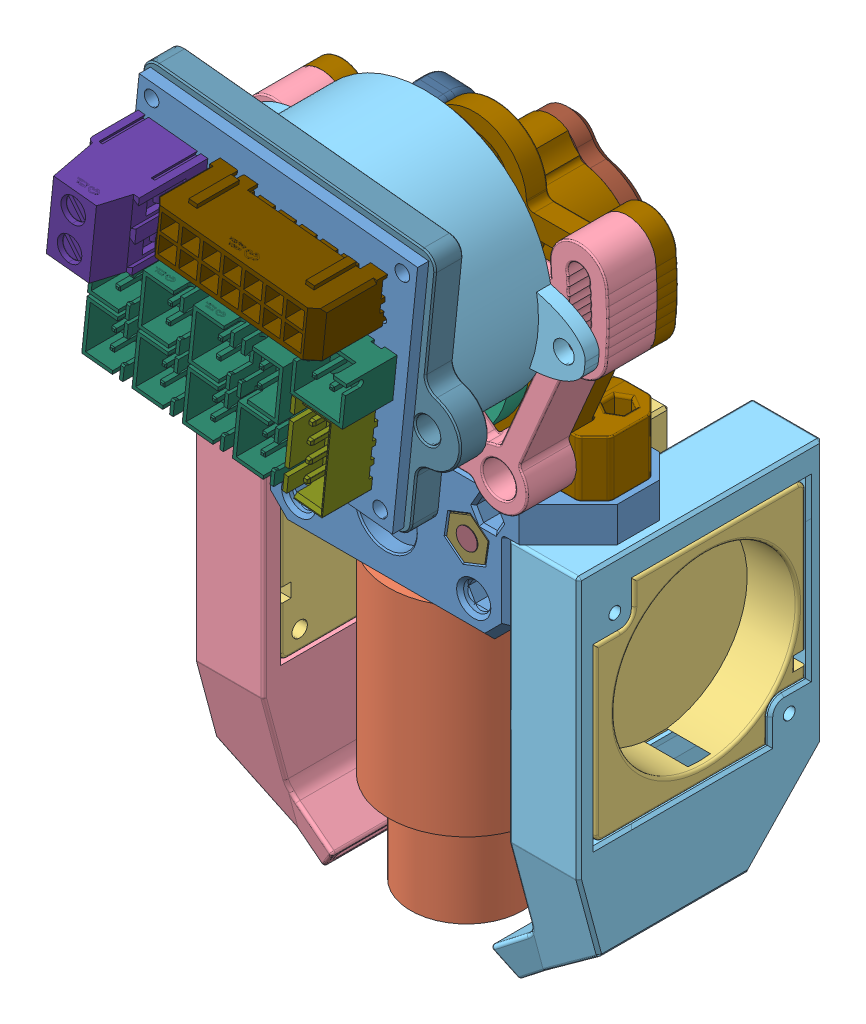
SolidWorks assembly TAP+换头-热端装配, configuration 默认. Lengths in mm.
Overall size (64.42 119.93 74.4).
63 component instances, 23 part files, 39 mates.
Components (placement in the parent):
- TAP+换头-V6固定座-1: TAP+换头-V6固定座 [Default] at (0.6992 -1.423 53.775) size (52 19.4 22.55)
- V6散热器-1: V6散热器 [Default] at (0.6992 1.577 53.775) x (-0.937959 0 -0.346747) z (-0.346747 0 0.937959) size (22.3 59 22.3)
- TAP+换头-V6固定座-1-1: TAP+换头-V6固定座-1 [Default] at (0.6992 -1.423 53.775) x (-1 0 0) z (0 0 -1) size (35 25.4 12.09)
- 挤出机组装-1: 挤出机组装 [Default] at (24.2197 76.008 94.8824) x (-1 0 0) z (0 -1 0) size (60.01 46.35 49.65)
  - 挤出机电机座-1: 挤出机电机座 [Default] at (-24.1653 27.1074 25.8748) size (56.72 7.01 44.47)
  - 36圆饼电机-1: 36圆饼电机 [Default] at (15.4671 9.6074 38.1257) x (0.994716 0 -0.102664) z (0.102664 0 0.994716) size (49.93 29 36.4)
  - BMG主齿组装-1: BMG主齿组装 [Default] at (16.3112 26.812 26.7681) x (0.995449 0 0.095298) z (-0.095298 0 0.995449) size (25.9 28.3 25.9)
    - BMG主齿-1: BMG主齿 [Default] at (5.4147 0.2954 24.6592) size (25.9 28.3 25.9)
    - BMG挤出齿-1: BMG挤出齿 [Default] at (5.4147 25.5954 24.6592) x (-0.887226 0 -0.461335) z (-0.461335 0 0.887226) size (9.4 14 9.4)
  - MR85-1: MR85 [Default] at (19.3513 27.6074 51.831) size (8 2.5 8)
  - 挤出机主体-1: 挤出机主体 [Default] at (-24.1653 34.1074 25.8748) size (59.44 18.3 40.97)
  - 挤出机从挤出齿轮支架-1: 挤出机从挤出齿轮支架 [Default] at (34.3823 55.9074 36.7653) x (0.043131 0 0.999069) z (0 -1 0) size (30 8.53 21.09)
  - BMG挤出齿-2: BMG挤出齿 [Default] at (28.0327 52.4074 51.9833) x (-0.837169 0 -0.546944) z (-0.546944 0 0.837169) size (9.4 14 9.4)
  - 挤出机盖子-1: 挤出机盖子 [Default] at (19.3513 55.9074 51.831) x (0.999977 0 0.006798) z (0.006798 0 -0.999977) size (25.23 3.5 27.46)
  - MR85-2: MR85 [Default] at (19.3513 54.9074 51.831) x (-0.837169 0 -0.546944) z (-0.546944 0 0.837169) size (8 2.5 8)
- M3螺母-1: M3螺母 [默认] at (12.1907 1.0199 62.875) x (-0.783317 0.621622 0) z (0.621622 0.783317 0) size (6.35 2.3 5.5)
- M3x20-1: M3x20 [Default] at (12.1992 1.077 65.275) x (-0.825766 -0.564012 0) z (0 0 -1) size (5.7 5.7 23)
- M3螺母-2: M3螺母 [默认] at (-10.8461 1.0411 62.875) x (-0.929999 0.367561 0) z (0.367561 0.929999 0) size (6.35 2.3 5.5)
- M3x20-2: M3x20 [Default] at (-10.8461 1.0411 65.275) x (-0.518434 0.855118 0) z (0 0 -1) size (5.7 5.7 23)
- PCB固定-2-2: PCB固定-2 [默认] at (-13.6764 25.1175 89.275) x (0.102664 0.994716 0) z (-0.994716 0.102664 0) size (37 4 53.35)
- 3D_HeadBoard_2024-03-10.step-1: 3D_HeadBoard_2024-03-10.step [默认] at (-8.9858 60.8247 89.275) x (0.994716 -0.102664 0) z (0 0 1) size (39.97 34.97 17.5)
  - FAN2.step-1: FAN2.step [默认] at (13.0535 -19.558 1.6001) x (0 -1 0) z (0 0 1) size (7.5 5.9 10.6)
    - CONN-TH_2P-P2.50_HX25003-2A.step-1: CONN-TH_2P-P2.50_HX25003-2A.step [默认] at origin size (7.5 5.9 10.6)
      - COMPOUND.step-1: COMPOUND.step [默认] at origin size (7.5 5.9 10.6)
  - PROBE.step-1: PROBE.step [默认] at (13.0535 -27.5591 1.6001) x (0 -1 0) z (0 0 1) size (7.5 5.9 10.6)
    - CONN-TH_2P-P2.50_HX25003-2A.step-1: CONN-TH_2P-P2.50_HX25003-2A.step [默认] at origin size (7.5 5.9 10.6)
      - COMPOUND.step-1: COMPOUND.step [默认] at origin size (7.5 5.9 10.6)
  - TEM1.step-1: TEM1.step [默认] at (27.4766 -27.5591 1.6001) x (0 -1 0) z (0 0 1) size (7.5 5.9 10.6)
    - CONN-TH_2P-P2.50_HX25003-2A.step-1: CONN-TH_2P-P2.50_HX25003-2A.step [默认] at origin size (7.5 5.9 10.6)
      - COMPOUND.step-1: COMPOUND.step [默认] at origin size (7.5 5.9 10.6)
  - TEM2.step-1: TEM2.step [默认] at (20.2651 -27.5591 1.6001) x (0 -1 0) z (0 0 1) size (7.5 5.9 10.6)
    - CONN-TH_2P-P2.50_HX25003-2A.step-1: CONN-TH_2P-P2.50_HX25003-2A.step [默认] at origin size (7.5 5.9 10.6)
      - COMPOUND.step-1: COMPOUND.step [默认] at origin size (7.5 5.9 10.6)
  - 5V.step-1: 5V.step [默认] at (34.6711 -14.859 1.6001) size (7.5 5.9 10.6)
    - CONN-TH_2P-P2.50_HX25003-2A.step-1: CONN-TH_2P-P2.50_HX25003-2A.step [默认] at origin size (7.5 5.9 10.6)
      - COMPOUND.step-1: COMPOUND.step [默认] at origin size (7.5 5.9 10.6)
  - FAN2-1.step-1: FAN2-1.step [默认] at (5.842 -19.558 1.6001) x (0 -1 0) z (0 0 1) size (7.5 5.9 10.6)
    - CONN-TH_2P-P2.50_HX25003-2A.step-1: CONN-TH_2P-P2.50_HX25003-2A.step [默认] at origin size (7.5 5.9 10.6)
      - COMPOUND.step-1: COMPOUND.step [默认] at origin size (7.5 5.9 10.6)
  - X-ENDSTOP.step-1: X-ENDSTOP.step [默认] at (5.842 -27.5591 1.6001) x (0 -1 0) z (0 0 1) size (7.5 5.9 10.6)
    - CONN-TH_2P-P2.50_HX25003-2A.step-1: CONN-TH_2P-P2.50_HX25003-2A.step [默认] at origin size (7.5 5.9 10.6)
      - COMPOUND.step-1: COMPOUND.step [默认] at origin size (7.5 5.9 10.6)
  - VCC.step-1: VCC.step [默认] at (26.1621 -19.558 1.6001) x (0 1 0) z (0 0 1) size (7.5 5.9 10.6)
    - CONN-TH_2P-P2.50_HX25003-2A.step-1: CONN-TH_2P-P2.50_HX25003-2A.step [默认] at origin size (7.5 5.9 10.6)
      - COMPOUND.step-1: COMPOUND.step [默认] at origin size (7.5 5.9 10.6)
  - FAN1.step-1: FAN1.step [默认] at (20.2651 -19.558 1.6001) x (0 -1 0) z (0 0 1) size (7.5 5.9 10.6)
    - CONN-TH_2P-P2.50_HX25003-2A.step-1: CONN-TH_2P-P2.50_HX25003-2A.step [默认] at origin size (7.5 5.9 10.6)
      - COMPOUND.step-1: COMPOUND.step [默认] at origin size (7.5 5.9 10.6)
  - E_MOTO.step-1: E_MOTO.step [默认] at (33.2741 -25.0864 1.6001) x (0 -1 0) z (0 0 1) size (12.5 5.7 10)
    - CONN-TH_4P-P2.50_4PIN.step-1: CONN-TH_4P-P2.50_4PIN.step [默认] at origin size (12.5 5.7 10)
      - COMPOUND-0.step-1: COMPOUND-0.step [默认] at origin size (12.5 5.7 10)
  - HOT.step-1: HOT.step [默认] at (5.842 -9.652 1.6001) x (0 1 0) z (0 0 1) size (10.76 10 17.5)
    - CONN-TH_2P-P5.00_WJ500V-5.08-2P.step-1: CONN-TH_2P-P5.00_WJ500V-5.08-2P.step [默认] at origin size (10.76 10 17.5)
      - COMPOUND-1.step-1: COMPOUND-1.step [默认] at origin size (10.76 10 17.5)
  - HEAD_IN.step-1: HEAD_IN.step [默认] at (24.003 -6.858 1.6001) x (-1 0 0) z (0 0 1) size (24 8.8 13.2)
    - CONN-TH_14P-P3.00_HC-MX3.0-2X7A.step-1: CONN-TH_14P-P3.00_HC-MX3.0-2X7A.step [默认] at origin size (24 8.8 13.2)
      - SOLID.step-1: SOLID.step [默认] at origin size (24 8.8 13.2)
  - COMPOUND-2.step-1: COMPOUND-2.step [默认] at origin size (39.97 34.97 1.6)
- 3010风扇-1: 3010风扇 [Default] at (-14.3008 -39.823 42.275) x (1 0 0) z (0 1 0) size (30 10 30)
- 3010涡轮-1: 3010涡轮 [Default] at (-16.8008 0.077 32.875) x (0 0 1) z (0 -1 0) size (30 10.07 30)
- V2吹料-1-1: V2吹料-1 [默认] at (-26.8008 0.077 65.275) size (16.15 60.54 34.8)
- 镜向V2吹料-1-2: 镜向V2吹料-1 [默认] at (28.1992 0.077 65.275) x (-1 0 0) z (0 0 -1) size (16.15 60.54 34.8)
- 3010涡轮-2: 3010涡轮 [Default] at (18.1992 0.077 62.875) x (0 0 -1) z (0 -1 0) size (30 10.07 30)
Mates (geometry in assembly coordinates):
- 重合1: coincident anti-aligned: plane of TAP+换头-V6固定座-1 through (0.6992 -1.423 53.775) normal (0 1 0); plane of V6散热器-1 through (0.6992 -1.423 53.775) normal (0 -1 0)
- 同心1: concentric aligned: cylinder of TAP+换头-V6固定座-1 through (0.6992 -10.323 53.775) axis (0 1 0) radius 8.05; cylinder of V6散热器-1 through (0.6992 -8.923 53.775) axis (0 1 0) radius 8
- 重合2: coincident aligned: plane of TAP+换头-V6固定座-1 through (0.6992 9.077 53.775) normal (0 1 0); plane of TAP+换头-V6固定座-1-1 through (0.6992 9.077 53.775) normal (0 1 0)
- 同心3: concentric anti-aligned: cylinder of V6散热器-1 through (0.6992 -8.923 53.775) axis (0 1 0) radius 8; cylinder of TAP+换头-V6固定座-1-1 through (0.6992 4.077 53.775) axis (0 -1 0) radius 8.05
- 平行1: parallel anti-aligned: plane of TAP+换头-V6固定座-1 through (0.6992 -1.423 65.275) normal (0 0 1); plane of TAP+换头-V6固定座-1-1 through (0.6992 -1.423 42.275) normal (0 0 -1)
- 重合4: coincident anti-aligned: plane of TAP+换头-V6固定座-1-1 through (0.6992 -1.423 42.275) normal (0 0 -1); plane of 3010风扇-1 through (-14.3008 -39.823 42.275) normal (0 0 1)
- 重合5: coincident anti-aligned: plane of TAP+换头-V6固定座-1 through (0.6992 9.077 53.775) normal (0 1 0); plane of 挤出机组装-1/挤出机主体-1 through (48.385 9.077 57.775) normal (0 -1 0)
- 重合6: coincident aligned: plane of TAP+换头-V6固定座-1 through (-1.3508 9.077 53.775) normal (1 0 0); plane of 挤出机组装-1/挤出机主体-1 through (-1.3508 19.077 54.9586) normal (1 0 0)
- 重合7: coincident aligned: plane of TAP+换头-V6固定座-1 through (-0.3258 9.077 55.5504) normal (0.5 0 -0.866025); plane of 挤出机组装-1/挤出机主体-1 through (0.6992 19.077 56.1421) normal (0.5 0 -0.866025)
- 重合8: coincident anti-aligned: plane of TAP+换头-V6固定座-1 through (11.7249 -2.1212 62.875) normal (-0.367561 0.929999 0); plane of M3螺母-1 through (11.7249 -2.1212 65.175) normal (0.367561 -0.929999 0)
- 重合9: coincident anti-aligned: plane of TAP+换头-V6固定座-1 through (0.6992 -1.423 62.875) normal (0 0 1); plane of M3螺母-1 through (12.1907 1.0199 62.875) normal (0 0 -1)
- 重合10: coincident anti-aligned: plane of TAP+换头-V6固定座-1 through (9.1923 -0.1114 62.875) normal (0.621622 0.783317 0); plane of M3螺母-1 through (9.2375 -0.1473 65.175) normal (-0.621622 -0.783317 0)
- 重合11: coincident anti-aligned: plane of TAP+换头-V6固定座-1 through (0.6992 -1.423 62.875) normal (0 0 1); plane of M3螺母-2 through (-10.8461 1.0411 62.875) normal (0 0 -1)
- 重合12: coincident anti-aligned: plane of TAP+换头-V6固定座-1 through (-13.8077 2.2654 62.875) normal (0.989184 0.146682 0); plane of M3螺母-2 through (-13.7992 2.2082 65.175) normal (-0.989184 -0.146682 0)
- 重合13: coincident anti-aligned: plane of TAP+换头-V6固定座-1 through (-13.3334 -0.9328 62.875) normal (0.367561 0.929999 0); plane of M3螺母-2 through (-13.3334 -0.9328 65.175) normal (-0.367561 -0.929999 0)
- 同心6: concentric anti-aligned: cylinder of TAP+换头-V6固定座-1-1 through (12.1992 1.077 53.675) axis (0 0 -1) radius 1.65; cylinder of M3x20-1 through (12.1992 1.077 45.275) axis (0 0 1) radius 1.5
- 同心7: concentric aligned: circle of TAP+换头-V6固定座-1-1; circle of M3x20-1
- 重合14: coincident aligned: plane of TAP+换头-V6固定座-1-1 through (0.6992 -1.423 42.275) normal (0 0 -1); plane of M3x20-1 through (12.1992 1.077 42.275) normal (0 0 -1)
- 重合15: coincident aligned: circle of M3螺母-2; cylinder of M3x20-2 through (-10.8461 1.0411 45.275) axis (0 0 1) radius 1.5
- 重合16: coincident aligned: plane of TAP+换头-V6固定座-1-1 through (0.6992 -1.423 42.275) normal (0 0 -1); plane of M3x20-2 through (-10.8461 1.0411 42.275) normal (0 0 -1)
- 重合17: coincident anti-aligned: plane of 挤出机组装-1/36圆饼电机-1 through (8.7526 37.8823 85.275) normal (0 0 1); plane of PCB固定-2-2 through (-13.6764 25.1175 85.275) normal (0 0 -1)
- 同心9: concentric anti-aligned: cylinder of 挤出机组装-1/36圆饼电机-1 through (30.5618 35.6314 69.775) axis (0 0 -1) radius 1.5; circle of PCB固定-2-2
- 同心10: concentric anti-aligned: cylinder of 挤出机组装-1/36圆饼电机-1 through (-13.0565 40.1332 69.775) axis (0 0 -1) radius 1.5; cylinder of PCB固定-2-2 through (-13.0565 40.1332 85.275) axis (0 0 1) radius 1.75
- 重合18: coincident anti-aligned: plane of PCB固定-2-2 through (-13.6764 25.1175 89.275) normal (0 0 1); plane of 3D_HeadBoard_2024-03-10.step-1/COMPOUND-2.step-1 through (9.1119 41.3638 89.275) normal (0 0 -1)
- 同心11: concentric aligned: cylinder of PCB固定-2-2 through (28.6081 54.934 85.275) axis (0 0 1) radius 0.85; cylinder of 3D_HeadBoard_2024-03-10.step-1/COMPOUND-2.step-1 through (28.6081 54.934 89.275) axis (0 0 1) radius 1.05
- 同心12: concentric aligned: cylinder of PCB固定-2-2 through (-10.3842 27.7937 85.275) axis (0 0 1) radius 0.85; cylinder of 3D_HeadBoard_2024-03-10.step-1/COMPOUND-2.step-1 through (-10.3843 27.7936 89.275) axis (0 0 1) radius 1.05
- 重合19: coincident anti-aligned: plane of TAP+换头-V6固定座-1-1 through (0.6992 -1.423 42.275) normal (0 0 -1); plane of 3010风扇-1 through (-14.3008 -39.823 42.275) normal (0 0 1)
- 同心13: concentric aligned: cylinder of TAP+换头-V6固定座-1-1 through (12.6992 -12.823 52.275) axis (0 0 -1) radius 1.5; cylinder of 3010风扇-1 through (12.6992 -12.823 42.275) axis (0 0 -1) radius 1.5
- 重合20: coincident aligned: circle of TAP+换头-V6固定座-1-1; cylinder of 3010风扇-1 through (-11.3008 -12.823 42.275) axis (0 0 -1) radius 1.5
- 重合21: coincident anti-aligned: plane of TAP+换头-V6固定座-1-1 through (-16.8008 -1.423 53.775) normal (-1 0 0); plane of 3010涡轮-1 through (-16.8008 0.077 32.875) normal (1 0 0)
- 平行3: parallel aligned: plane of V6散热器-1 through (0.6992 -39.423 53.775) normal (0 -1 0); plane of 3010涡轮-1 through (-16.8008 -27.923 32.875) normal (0 -1 0)
- 重合25: coincident anti-aligned: plane of TAP+换头-V6固定座-1 through (0.6992 4.077 53.775) normal (0 -1 0); plane of V2吹料-1-1 through (-26.8008 4.077 65.275) normal (0 1 0)
- 重合27: coincident anti-aligned: plane of 3010涡轮-1 through (-26.8008 0.077 32.875) normal (0 1 0); plane of V2吹料-1-1 through (-26.8008 0.077 65.275) normal (0 -1 0)
- 重合28: coincident anti-aligned: plane of 3010涡轮-1 through (-26.8008 0.077 62.875) normal (0 0 1); plane of V2吹料-1-1 through (-26.8008 -30.323 62.875) normal (0 0 -1)
- 重合29: coincident anti-aligned: plane of TAP+换头-V6固定座-1 through (-16.8008 -1.423 53.775) normal (-1 0 0); plane of V2吹料-1-1 through (-16.8008 4.077 65.275) normal (1 0 0)
- 重合30: coincident aligned: plane of TAP+换头-V6固定座-1 through (0.6992 -1.423 65.275) normal (0 0 1); plane of V2吹料-1-1 through (-26.8008 4.077 65.275) normal (0 0 1)
- 重合31: coincident aligned: plane of 镜向V2吹料-1-2 through (18.1992 4.077 65.275) normal (-1 0 0); plane of 3010涡轮-2 through (18.1992 0.077 62.875) normal (-1 0 0)
- 重合32: coincident anti-aligned: plane of 镜向V2吹料-1-2 through (28.1992 0.077 65.275) normal (0 -1 0); plane of 3010涡轮-2 through (28.1992 0.077 62.875) normal (0 1 0)
- 重合33: coincident anti-aligned: plane of 镜向V2吹料-1-2 through (28.1992 -30.323 62.875) normal (0 0 -1); plane of 3010涡轮-2 through (28.1992 0.077 62.875) normal (0 0 1)
